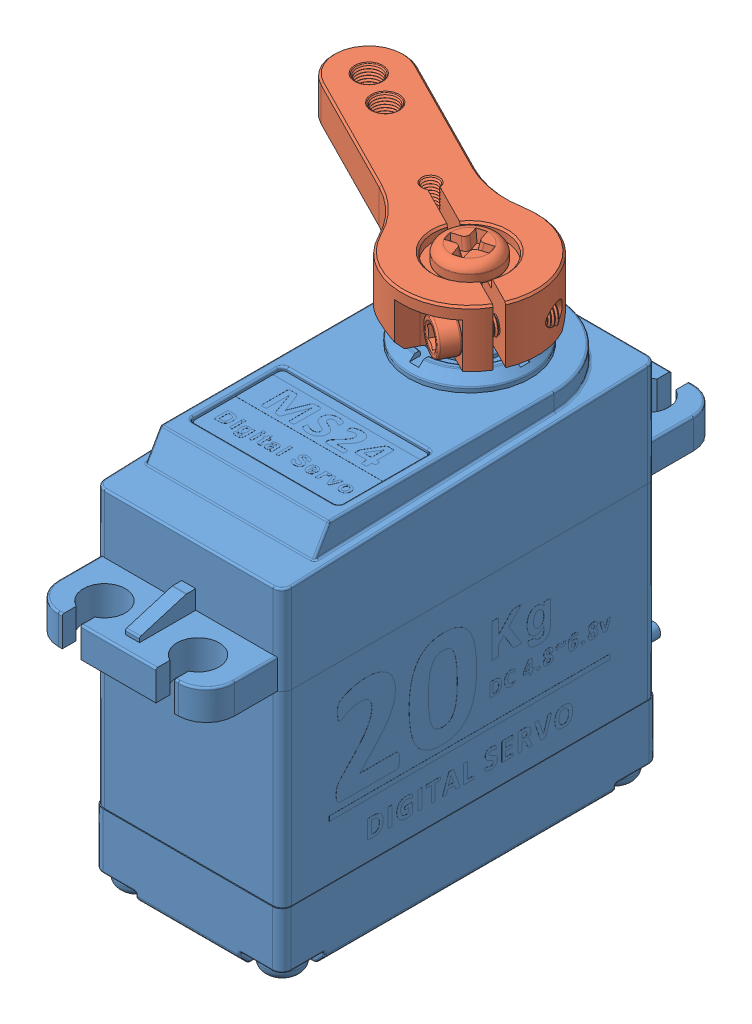
SolidWorks assembly DS3240 Digital Servo, configuration Default. Lengths in mm.
Overall size (38.57 49.37 56.76).
2 component instances, 2 part files, 2 mates.
Components (placement in the parent):
- DS3218MG MS24 Digital Servo 270^DS3240 Digital Servo-1: DS3218MG MS24 Digital Servo 270^DS3240 Digital Servo [Default] at origin size (20.1 45.99 55.6) (virtual)
- Servo Arm^DS3240 Digital Servo-1: Servo Arm^DS3240 Digital Servo [Default] x (0.452122 0 -0.891956) z (0.891956 0 0.452122) size (14.5 6.95 35.53) (virtual)
Mates (geometry in assembly coordinates):
- Concentric1: concentric anti-aligned: cylinder of Servo Arm^DS3240 Digital Servo-1 through (0 18.4 0) axis (0 -1 0) radius 2.5; cylinder of DS3218MG MS24 Digital Servo 270-1 through (0 13.5 0) axis (0 1 0) radius 3.8
- Coincident1: coincident anti-aligned: plane of Copy of DS3218MG MS24 Digital Servo 270^DS3240 Digital Servo-1 through (0 18.4 0) normal (0 1 0); plane of Servo Arm^DS3240 Digital Servo-1 through (0 18.4 0) normal (0 -1 0)
